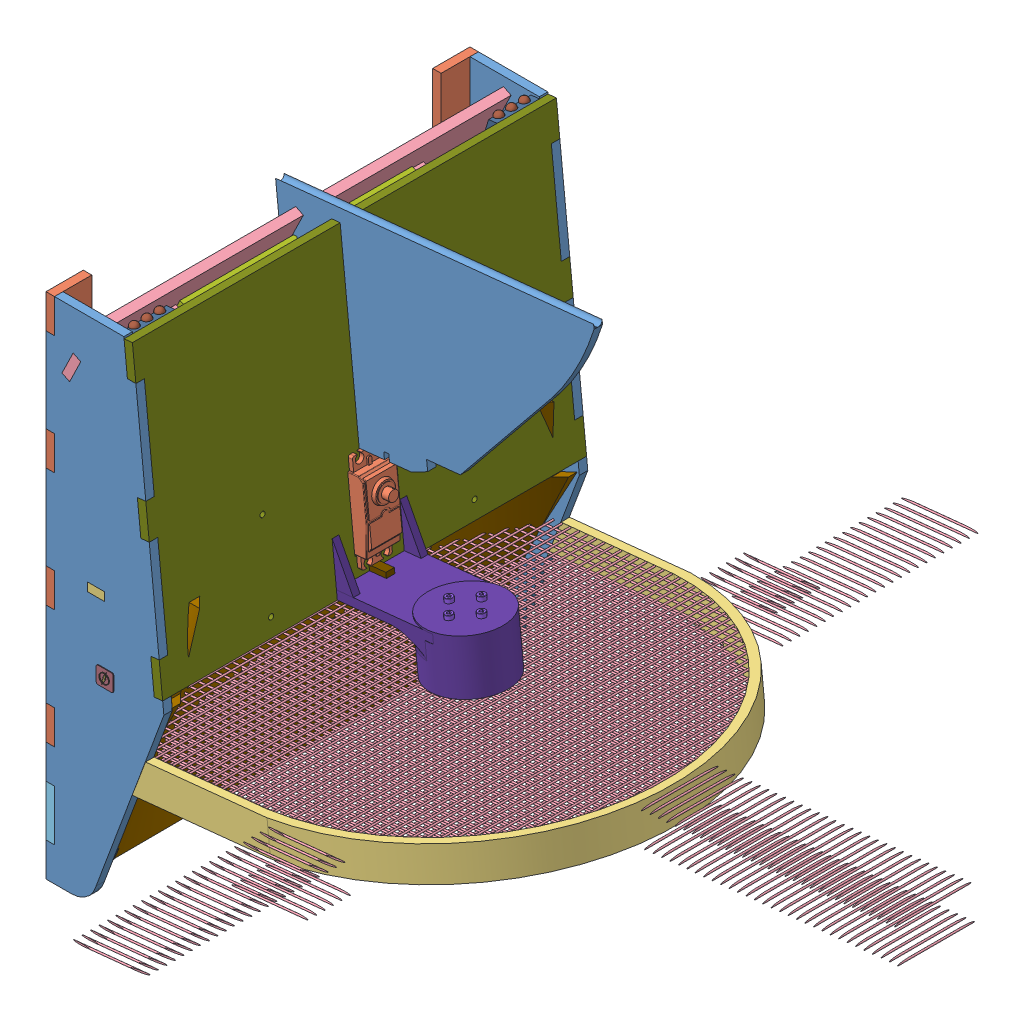
SolidWorks assembly AssStructSimu, configuration Défaut. Lengths in mm. (continued)
Components (placement in the parent): (continued)
- AssCarte-1: AssCarte [Défaut] at (38.0121 147.1029 290.772) x (-0.101852 0.9948 0) z (0.9948 0.101852 0) size (66.52 130.57 98.72) (hidden) (continued)
  - carte_onduleur_v3-1: carte_onduleur_v3 [Défaut] at (-131.8199 12.0892 20.7912) size (66.52 130.57 82.34) (continued)
    - C_DEC_COMP3-1: C_DEC_COMP3 [Défaut] at (-14.6 -22.9 0.803) x (0 -1 0) z (0 0 1) size (2.34 1.04 0.5) (continued)
      - Open CASCADE STEP translator 6.8 1.6.1-1: Open CASCADE STEP translator 6.8 1.6.1 [Défaut] at origin size (2.34 1.04 0.5) (continued)
        - Pin_2-1: Pin_2 [Défaut] at origin size (0.51 1.02 0.5)
    - D_VBAT-1: D_VBAT [Défaut] at (-1.2 46.4 0.803) x (0 -1 0) z (0 0 1) size (2.34 1.04 0.5)
      - Open CASCADE STEP translator 6.8 1.6.1-1: Open CASCADE STEP translator 6.8 1.6.1 [Défaut] at origin size (2.34 1.04 0.5)
        - Body_1-1: Body_1 [Défaut] at origin size (2.29 1.04 0.43)
        - Pin_1-1: Pin_1 [Défaut] at (0.3048 0 0) x (-1 0 0) z (0 0 1) size (0.51 1.02 0.5)
        - Pin_2-1: Pin_2 [Défaut] at origin size (0.51 1.02 0.5)
    - D_3V-1: D_3V [Défaut] at (1.3 46.3 0.803) x (0 -1 0) z (0 0 1) size (2.34 1.04 0.5)
      - Open CASCADE STEP translator 6.8 1.6.1-1: Open CASCADE STEP translator 6.8 1.6.1 [Défaut] at origin size (2.34 1.04 0.5)
        - Body_1-1: Body_1 [Défaut] at origin size (2.29 1.04 0.43)
        - Pin_1-1: Pin_1 [Défaut] at (0.3048 0 0) x (-1 0 0) z (0 0 1) size (0.51 1.02 0.5)
        - Pin_2-1: Pin_2 [Défaut] at origin size (0.51 1.02 0.5)
    - D_5V-1: D_5V [Défaut] at (-3.7 46.4 0.803) x (0 -1 0) z (0 0 1) size (2.34 1.04 0.5)
      - Open CASCADE STEP translator 6.8 1.6.1-1: Open CASCADE STEP translator 6.8 1.6.1 [Défaut] at origin size (2.34 1.04 0.5)
        - Body_1-1: Body_1 [Défaut] at origin size (2.29 1.04 0.43)
        - Pin_1-1: Pin_1 [Défaut] at (0.3048 0 0) x (-1 0 0) z (0 0 1) size (0.51 1.02 0.5)
        - Pin_2-1: Pin_2 [Défaut] at origin size (0.51 1.02 0.5)
    - R1_1-1: R1_1 [Défaut] at (-20.2 -36.1 0.803) x (-1 0 0) z (0 0 1) size (2.34 1.04 0.5)
      - Open CASCADE STEP translator 6.8 1.12.1-1: Open CASCADE STEP translator 6.8 1.12.1 [Défaut] at origin size (2.34 1.04 0.5)
        - Body_1_3-1: Body_1_3 [Défaut] at origin size (2.29 1.04 0.43)
        - Pin_1_2-1: Pin_1_2 [Défaut] at (0.3048 0 0) x (-1 0 0) z (0 0 1) size (0.51 1.02 0.5)
        - Pin_2_2-1: Pin_2_2 [Défaut] at origin size (0.51 1.02 0.5)
    - R1_2-1: R1_2 [Défaut] at (-15.5 -34.6 0.803) x (-1 0 0) z (0 0 1) size (2.34 1.04 0.5)
      - Open CASCADE STEP translator 6.8 1.12.1-1: Open CASCADE STEP translator 6.8 1.12.1 [Défaut] at origin size (2.34 1.04 0.5)
        - Body_1_3-1: Body_1_3 [Défaut] at origin size (2.29 1.04 0.43)
        - Pin_1_2-1: Pin_1_2 [Défaut] at (0.3048 0 0) x (-1 0 0) z (0 0 1) size (0.51 1.02 0.5)
        - Pin_2_2-1: Pin_2_2 [Défaut] at origin size (0.51 1.02 0.5)
    - R1_3-1: R1_3 [Défaut] at (-20.3 -39.9 0.803) x (-1 0 0) z (0 0 1) size (2.34 1.04 0.5)
      - Open CASCADE STEP translator 6.8 1.12.1-1: Open CASCADE STEP translator 6.8 1.12.1 [Défaut] at origin size (2.34 1.04 0.5)
        - Body_1_3-1: Body_1_3 [Défaut] at origin size (2.29 1.04 0.43)
        - Pin_1_2-1: Pin_1_2 [Défaut] at (0.3048 0 0) x (-1 0 0) z (0 0 1) size (0.51 1.02 0.5)
        - Pin_2_2-1: Pin_2_2 [Défaut] at origin size (0.51 1.02 0.5)
    - R1_4-1: R1_4 [Défaut] at (-20.3 -38.1 0.803) x (-1 0 0) z (0 0 1) size (2.34 1.04 0.5)
      - Open CASCADE STEP translator 6.8 1.12.1-1: Open CASCADE STEP translator 6.8 1.12.1 [Défaut] at origin size (2.34 1.04 0.5)
        - Body_1_3-1: Body_1_3 [Défaut] at origin size (2.29 1.04 0.43)
        - Pin_1_2-1: Pin_1_2 [Défaut] at (0.3048 0 0) x (-1 0 0) z (0 0 1) size (0.51 1.02 0.5)
        - Pin_2_2-1: Pin_2_2 [Défaut] at origin size (0.51 1.02 0.5)
    - R1_5-1: R1_5 [Défaut] at (-17.1336 -39.7 0.803) size (2.34 1.04 0.5)
      - Open CASCADE STEP translator 6.8 1.12.1-1: Open CASCADE STEP translator 6.8 1.12.1 [Défaut] at origin size (2.34 1.04 0.5)
        - Body_1_3-1: Body_1_3 [Défaut] at origin size (2.29 1.04 0.43)
        - Pin_1_2-1: Pin_1_2 [Défaut] at (0.3048 0 0) x (-1 0 0) z (0 0 1) size (0.51 1.02 0.5)
        - Pin_2_2-1: Pin_2_2 [Défaut] at origin size (0.51 1.02 0.5)
    - R2_1-1: R2_1 [Défaut] at (-18.5 -9.5 0.803) x (-1 0 0) z (0 0 1) size (2.34 1.04 0.5)
      - Open CASCADE STEP translator 6.8 1.12.1-1: Open CASCADE STEP translator 6.8 1.12.1 [Défaut] at origin size (2.34 1.04 0.5)
        - Body_1_3-1: Body_1_3 [Défaut] at origin size (2.29 1.04 0.43)
        - Pin_1_2-1: Pin_1_2 [Défaut] at (0.3048 0 0) x (-1 0 0) z (0 0 1) size (0.51 1.02 0.5)
        - Pin_2_2-1: Pin_2_2 [Défaut] at origin size (0.51 1.02 0.5)
    - R2_2-1: R2_2 [Défaut] at (-13.1 -8 0.803) x (-1 0 0) z (0 0 1) size (2.34 1.04 0.5)
      - Open CASCADE STEP translator 6.8 1.12.1-1: Open CASCADE STEP translator 6.8 1.12.1 [Défaut] at origin size (2.34 1.04 0.5)
        - Body_1_3-1: Body_1_3 [Défaut] at origin size (2.29 1.04 0.43)
        - Pin_1_2-1: Pin_1_2 [Défaut] at (0.3048 0 0) x (-1 0 0) z (0 0 1) size (0.51 1.02 0.5)
        - Pin_2_2-1: Pin_2_2 [Défaut] at origin size (0.51 1.02 0.5)
    - R2_3-1: R2_3 [Défaut] at (-18.5 -11.2 0.803) x (-1 0 0) z (0 0 1) size (2.34 1.04 0.5)
      - Open CASCADE STEP translator 6.8 1.12.1-1: Open CASCADE STEP translator 6.8 1.12.1 [Défaut] at origin size (2.34 1.04 0.5)
        - Body_1_3-1: Body_1_3 [Défaut] at origin size (2.29 1.04 0.43)
        - Pin_1_2-1: Pin_1_2 [Défaut] at (0.3048 0 0) x (-1 0 0) z (0 0 1) size (0.51 1.02 0.5)
        - Pin_2_2-1: Pin_2_2 [Défaut] at origin size (0.51 1.02 0.5)
    - R2_4-1: R2_4 [Défaut] at (-18.5 -12.8 0.803) x (-1 0 0) z (0 0 1) size (2.34 1.04 0.5)
      - Open CASCADE STEP translator 6.8 1.12.1-1: Open CASCADE STEP translator 6.8 1.12.1 [Défaut] at origin size (2.34 1.04 0.5)
        - Body_1_3-1: Body_1_3 [Défaut] at origin size (2.29 1.04 0.43)
        - Pin_1_2-1: Pin_1_2 [Défaut] at (0.3048 0 0) x (-1 0 0) z (0 0 1) size (0.51 1.02 0.5)
        - Pin_2_2-1: Pin_2_2 [Défaut] at origin size (0.51 1.02 0.5)
    - R2_5-1: R2_5 [Défaut] at (-15.1336 -13 0.803) size (2.34 1.04 0.5)
      - Open CASCADE STEP translator 6.8 1.12.1-1: Open CASCADE STEP translator 6.8 1.12.1 [Défaut] at origin size (2.34 1.04 0.5)
        - Body_1_3-1: Body_1_3 [Défaut] at origin size (2.29 1.04 0.43)
        - Pin_1_2-1: Pin_1_2 [Défaut] at (0.3048 0 0) x (-1 0 0) z (0 0 1) size (0.51 1.02 0.5)
        - Pin_2_2-1: Pin_2_2 [Défaut] at origin size (0.51 1.02 0.5)
    - R3_1-1: R3_1 [Défaut] at (-19.9 -23.1 0.803) x (-1 0 0) z (0 0 1) size (2.34 1.04 0.5)
      - Open CASCADE STEP translator 6.8 1.12.1-1: Open CASCADE STEP translator 6.8 1.12.1 [Défaut] at origin size (2.34 1.04 0.5)
        - Body_1_3-1: Body_1_3 [Défaut] at origin size (2.29 1.04 0.43)
        - Pin_1_2-1: Pin_1_2 [Défaut] at (0.3048 0 0) x (-1 0 0) z (0 0 1) size (0.51 1.02 0.5)
        - Pin_2_2-1: Pin_2_2 [Défaut] at origin size (0.51 1.02 0.5)
    - R3_2-1: R3_2 [Défaut] at (-14.7 -21.6 0.803) x (-1 0 0) z (0 0 1) size (2.34 1.04 0.5)
      - Open CASCADE STEP translator 6.8 1.12.1-1: Open CASCADE STEP translator 6.8 1.12.1 [Défaut] at origin size (2.34 1.04 0.5)
        - Body_1_3-1: Body_1_3 [Défaut] at origin size (2.29 1.04 0.43)
        - Pin_1_2-1: Pin_1_2 [Défaut] at (0.3048 0 0) x (-1 0 0) z (0 0 1) size (0.51 1.02 0.5)
        - Pin_2_2-1: Pin_2_2 [Défaut] at origin size (0.51 1.02 0.5)
    - R3_3-1: R3_3 [Défaut] at (-19.9 -24.8 0.803) x (-1 0 0) z (0 0 1) size (2.34 1.04 0.5)
      - Open CASCADE STEP translator 6.8 1.12.1-1: Open CASCADE STEP translator 6.8 1.12.1 [Défaut] at origin size (2.34 1.04 0.5)
        - Body_1_3-1: Body_1_3 [Défaut] at origin size (2.29 1.04 0.43)
        - Pin_1_2-1: Pin_1_2 [Défaut] at (0.3048 0 0) x (-1 0 0) z (0 0 1) size (0.51 1.02 0.5)
        - Pin_2_2-1: Pin_2_2 [Défaut] at origin size (0.51 1.02 0.5)
    - R3_4-1: R3_4 [Défaut] at (-19.9 -26.4 0.803) x (-1 0 0) z (0 0 1) size (2.34 1.04 0.5)
      - Open CASCADE STEP translator 6.8 1.12.1-1: Open CASCADE STEP translator 6.8 1.12.1 [Défaut] at origin size (2.34 1.04 0.5)
        - Body_1_3-1: Body_1_3 [Défaut] at origin size (2.29 1.04 0.43)
        - Pin_1_2-1: Pin_1_2 [Défaut] at (0.3048 0 0) x (-1 0 0) z (0 0 1) size (0.51 1.02 0.5)
        - Pin_2_2-1: Pin_2_2 [Défaut] at origin size (0.51 1.02 0.5)
    - R3_5-1: R3_5 [Défaut] at (-16.7336 -26.5 0.803) size (2.34 1.04 0.5)
      - Open CASCADE STEP translator 6.8 1.12.1-1: Open CASCADE STEP translator 6.8 1.12.1 [Défaut] at origin size (2.34 1.04 0.5)
        - Body_1_3-1: Body_1_3 [Défaut] at origin size (2.29 1.04 0.43)
        - Pin_1_2-1: Pin_1_2 [Défaut] at (0.3048 0 0) x (-1 0 0) z (0 0 1) size (0.51 1.02 0.5)
        - Pin_2_2-1: Pin_2_2 [Défaut] at origin size (0.51 1.02 0.5)
    - R_LED_3V3-1: R_LED_3V3 [Défaut] at (1.3 47.9 0.803) x (0 1 0) z (0 0 1) size (2.34 1.04 0.5)
      - Open CASCADE STEP translator 6.8 1.12.1-1: Open CASCADE STEP translator 6.8 1.12.1 [Défaut] at origin size (2.34 1.04 0.5)
        - Body_1_3-1: Body_1_3 [Défaut] at origin size (2.29 1.04 0.43)
        - Pin_1_2-1: Pin_1_2 [Défaut] at (0.3048 0 0) x (-1 0 0) z (0 0 1) size (0.51 1.02 0.5)
        - Pin_2_2-1: Pin_2_2 [Défaut] at origin size (0.51 1.02 0.5)
    - R_LED_5V-1: R_LED_5V [Défaut] at (-3.7 47.7 0.803) x (0 1 0) z (0 0 1) size (2.34 1.04 0.5)
      - Open CASCADE STEP translator 6.8 1.12.1-1: Open CASCADE STEP translator 6.8 1.12.1 [Défaut] at origin size (2.34 1.04 0.5)
        - Body_1_3-1: Body_1_3 [Défaut] at origin size (2.29 1.04 0.43)
        - Pin_1_2-1: Pin_1_2 [Défaut] at (0.3048 0 0) x (-1 0 0) z (0 0 1) size (0.51 1.02 0.5)
        - Pin_2_2-1: Pin_2_2 [Défaut] at origin size (0.51 1.02 0.5)
    - R_LED_VBAT-1: R_LED_VBAT [Défaut] at (-1.2 47.9 0.803) x (0 1 0) z (0 0 1) size (2.34 1.04 0.5)
      - Open CASCADE STEP translator 6.8 1.12.1-1: Open CASCADE STEP translator 6.8 1.12.1 [Défaut] at origin size (2.34 1.04 0.5)
        - Body_1_3-1: Body_1_3 [Défaut] at origin size (2.29 1.04 0.43)
        - Pin_1_2-1: Pin_1_2 [Défaut] at (0.3048 0 0) x (-1 0 0) z (0 0 1) size (0.51 1.02 0.5)
        - Pin_2_2-1: Pin_2_2 [Défaut] at origin size (0.51 1.02 0.5)
  - AssEntretoise-1: AssEntretoise [Défaut] at (-156.8199 -51.2976 37.1344) x (0 0 -1) z (1 0 0) size (58.24 7.29 7.81)
    - socket head cap screw 4762_din-1: socket head cap screw 4762_din [EN ISO 4762 M3 x 5 - 5N] at (-2.4967 0.5867 0) size (8 5.5 5.5)
    - hexagonal_spacer_MF_M3_H20_HEX5.5_FTD6_MTL6-1: hexagonal_spacer_MF_M3_H20_HEX5.5_FTD6_MTL6 [Défaut] at (48.3433 0.5867 0) x (0 0 1) z (-1 0 0) size (6.36 5.51 26)
    - hex nut style 1 gradeab_din-1: hex nut style 1 gradeab_din [Hexagon Nut ISO 4032 - M3 - W - N] at (53.3433 0.5867 0) x (0 0.943962 0.330053) z (-1 0 0) size (5.5 6.35 2.4)
    - hexagonal_spacer_MF_M3_H12_HEX5.5_FTD6_MTL6-2: hexagonal_spacer_MF_M3_H12_HEX5.5_FTD6_MTL6 [Défaut] at (27.0633 0.5867 0) x (0 0.248308 0.968681) z (-1 0 0) size (6.36 5.51 18)
    - hexagonal_spacer_MF_M3_H12_HEX5.5_FTD6_MTL6-3: hexagonal_spacer_MF_M3_H12_HEX5.5_FTD6_MTL6 [Défaut] at (13.7833 0.5867 0) x (0 0 1) z (-1 0 0) size (6.36 5.51 18)
  - AssEntretoise-2: AssEntretoise [Défaut] at (-156.8199 68.7024 37.1344) x (0 0 -1) z (1 0 0) size (58.24 7.29 7.81)
    - socket head cap screw 4762_din-1: socket head cap screw 4762_din [EN ISO 4762 M3 x 5 - 5N] at (-2.4967 0.5867 0) size (8 5.5 5.5)
    - hexagonal_spacer_MF_M3_H20_HEX5.5_FTD6_MTL6-1: hexagonal_spacer_MF_M3_H20_HEX5.5_FTD6_MTL6 [Défaut] at (48.3433 0.5867 0) x (0 0 1) z (-1 0 0) size (6.36 5.51 26)
    - hex nut style 1 gradeab_din-1: hex nut style 1 gradeab_din [Hexagon Nut ISO 4032 - M3 - W - N] at (53.3433 0.5867 0) x (0 0.943962 0.330053) z (-1 0 0) size (5.5 6.35 2.4)
    - hexagonal_spacer_MF_M3_H12_HEX5.5_FTD6_MTL6-2: hexagonal_spacer_MF_M3_H12_HEX5.5_FTD6_MTL6 [Défaut] at (27.0633 0.5867 0) x (0 0.248308 0.968681) z (-1 0 0) size (6.36 5.51 18)
    - hexagonal_spacer_MF_M3_H12_HEX5.5_FTD6_MTL6-3: hexagonal_spacer_MF_M3_H12_HEX5.5_FTD6_MTL6 [Défaut] at (13.7833 0.5867 0) x (0 0 1) z (-1 0 0) size (6.36 5.51 18)
  - AssEntretoise-3: AssEntretoise [Défaut] at (-106.8199 -51.2976 37.1344) x (0 0 -1) z (1 0 0) size (58.24 7.29 7.81)
    - socket head cap screw 4762_din-1: socket head cap screw 4762_din [EN ISO 4762 M3 x 5 - 5N] at (-2.4967 0.5867 0) size (8 5.5 5.5)
    - hexagonal_spacer_MF_M3_H20_HEX5.5_FTD6_MTL6-1: hexagonal_spacer_MF_M3_H20_HEX5.5_FTD6_MTL6 [Défaut] at (48.3433 0.5867 0) x (0 0 1) z (-1 0 0) size (6.36 5.51 26)
    - hex nut style 1 gradeab_din-1: hex nut style 1 gradeab_din [Hexagon Nut ISO 4032 - M3 - W - N] at (53.3433 0.5867 0) x (0 0.943962 0.330053) z (-1 0 0) size (5.5 6.35 2.4)
    - hexagonal_spacer_MF_M3_H12_HEX5.5_FTD6_MTL6-2: hexagonal_spacer_MF_M3_H12_HEX5.5_FTD6_MTL6 [Défaut] at (27.0633 0.5867 0) x (0 0.248308 0.968681) z (-1 0 0) size (6.36 5.51 18)
    - hexagonal_spacer_MF_M3_H12_HEX5.5_FTD6_MTL6-3: hexagonal_spacer_MF_M3_H12_HEX5.5_FTD6_MTL6 [Défaut] at (13.7833 0.5867 0) x (0 0 1) z (-1 0 0) size (6.36 5.51 18)
  - AssEntretoise-4: AssEntretoise [Défaut] at (-106.8199 68.7024 37.1344) x (0 0 -1) z (1 0 0) size (58.24 7.29 7.81)
    - socket head cap screw 4762_din-1: socket head cap screw 4762_din [EN ISO 4762 M3 x 5 - 5N] at (-2.4967 0.5867 0) size (8 5.5 5.5)
    - hexagonal_spacer_MF_M3_H20_HEX5.5_FTD6_MTL6-1: hexagonal_spacer_MF_M3_H20_HEX5.5_FTD6_MTL6 [Défaut] at (48.3433 0.5867 0) x (0 0 1) z (-1 0 0) size (6.36 5.51 26)
    - hex nut style 1 gradeab_din-1: hex nut style 1 gradeab_din [Hexagon Nut ISO 4032 - M3 - W - N] at (53.3433 0.5867 0) x (0 0.943962 0.330053) z (-1 0 0) size (5.5 6.35 2.4)
    - hexagonal_spacer_MF_M3_H12_HEX5.5_FTD6_MTL6-2: hexagonal_spacer_MF_M3_H12_HEX5.5_FTD6_MTL6 [Défaut] at (27.0633 0.5867 0) x (0 0.248308 0.968681) z (-1 0 0) size (6.36 5.51 18)
    - hexagonal_spacer_MF_M3_H12_HEX5.5_FTD6_MTL6-3: hexagonal_spacer_MF_M3_H12_HEX5.5_FTD6_MTL6 [Défaut] at (13.7833 0.5867 0) x (0 0 1) z (-1 0 0) size (6.36 5.51 18)
  - AssMpu-1: AssMpu [Défaut] at (-150.6881 40.5798 29.6372) x (0.908747 0.417347 0) z (0 0 1) size (8 8 22.28)
    - hex nut style 1 gradeab_din-1: hex nut style 1 gradeab_din [Hexagon Nut ISO 4032 - M3 - W - N] at (0.2783 0.3227 1.2) size (5.5 6.35 2.4)
    - plain washer 6903 type ab_din-1: plain washer 6903 type ab_din [DIN 6903-A3] at (0.2783 0.3227 1.2) x (0 0 1) z (-1 0 0) size (1 8 8)
    - socket head cap screw 4762_din-1: socket head cap screw 4762_din [EN ISO 4762 M3 x 5 - 5N] at (0.2783 0.3227 19.76) x (0 0 -1) z (-0.852155 0.523289 0) size (8 5.5 5.5)
    - hexagonal_spacer_MF_M3_H12_HEX5.5_FTD6_MTL6-1: hexagonal_spacer_MF_M3_H12_HEX5.5_FTD6_MTL6 [Défaut] at (0.2783 0.3227 3.48) size (6.36 5.51 18)
  - AssMpu-2: AssMpu [Défaut] at (-130.3481 40.6665 29.6372) size (8 8 22.28)
    - hex nut style 1 gradeab_din-1: hex nut style 1 gradeab_din [Hexagon Nut ISO 4032 - M3 - W - N] at (0.2783 0.3227 1.2) size (5.5 6.35 2.4)
    - plain washer 6903 type ab_din-1: plain washer 6903 type ab_din [DIN 6903-A3] at (0.2783 0.3227 1.2) x (0 0 1) z (-1 0 0) size (1 8 8)
    - socket head cap screw 4762_din-1: socket head cap screw 4762_din [EN ISO 4762 M3 x 5 - 5N] at (0.2783 0.3227 19.76) x (0 0 -1) z (-0.852155 0.523289 0) size (8 5.5 5.5)
    - hexagonal_spacer_MF_M3_H12_HEX5.5_FTD6_MTL6-1: hexagonal_spacer_MF_M3_H12_HEX5.5_FTD6_MTL6 [Défaut] at (0.2783 0.3227 3.48) size (6.36 5.51 18)
  - AssCosse-1: AssCosse [Défaut] at (-142.6764 26.8797 71.168) x (0 -1 0) z (-0.344896 0 -0.938641) size (9.83 18.66 11.64)
    - socket head cap screw 4762_din-1: socket head cap screw 4762_din [EN ISO 4762 M3 x 6 - 6N] at (-5.1064 0.3659 0) size (9 5.5 5.5)
    - plain washer 6903 type ab_din-1: plain washer 6903 type ab_din [DIN 6903-A3] at (-2.1064 0.3659 0) size (1 8 8)
    - hex nut style 1 gradeab_din-2: hex nut style 1 gradeab_din [Hexagon Nut ISO 4032 - M3 - W - N] at (1.281 0.3659 0) x (0 0.924225 0.381849) z (-1 0 0) size (5.5 6.35 2.4)
    - 31880-1: 31880 [Default] at (0.4936 0.3659 0) x (0 0.344896 -0.938641) z (0 -0.938641 -0.344896) size (5.54 5 17.37)
  - AssCosse-2: AssCosse [Défaut] at (-142.6764 -2.9203 71.168) x (0 -1 0) z (-0.344896 0 -0.938641) size (9.83 18.66 11.64)
    - socket head cap screw 4762_din-1: socket head cap screw 4762_din [EN ISO 4762 M3 x 6 - 6N] at (-5.1064 0.3659 0) size (9 5.5 5.5)
    - plain washer 6903 type ab_din-1: plain washer 6903 type ab_din [DIN 6903-A3] at (-2.1064 0.3659 0) size (1 8 8)
    - hex nut style 1 gradeab_din-2: hex nut style 1 gradeab_din [Hexagon Nut ISO 4032 - M3 - W - N] at (1.281 0.3659 0) x (0 0.924225 0.381849) z (-1 0 0) size (5.5 6.35 2.4)
    - 31880-1: 31880 [Default] at (0.4936 0.3659 0) x (0 0.344896 -0.938641) z (0 -0.938641 -0.344896) size (5.54 5 17.37)
  - AssCosse-3: AssCosse [Défaut] at (-142.6764 12.0797 71.168) x (0 -1 0) z (-0.344896 0 -0.938641) size (9.83 18.66 11.64)
    - socket head cap screw 4762_din-1: socket head cap screw 4762_din [EN ISO 4762 M3 x 6 - 6N] at (-5.1064 0.3659 0) size (9 5.5 5.5)
    - plain washer 6903 type ab_din-1: plain washer 6903 type ab_din [DIN 6903-A3] at (-2.1064 0.3659 0) size (1 8 8)
    - hex nut style 1 gradeab_din-2: hex nut style 1 gradeab_din [Hexagon Nut ISO 4032 - M3 - W - N] at (1.281 0.3659 0) x (0 0.924225 0.381849) z (-1 0 0) size (5.5 6.35 2.4)
    - 31880-1: 31880 [Default] at (0.4936 0.3659 0) x (0 0.344896 -0.938641) z (0 -0.938641 -0.344896) size (5.54 5 17.37)
  - Terminal_QD_Female-1: Terminal_QD_Female [Default] at (-137.2199 31.5422 53.3942) x (0 1 0) z (-1 0 0) size (9.4 5.5 22.35)
  - Terminal_QD_Female-2: Terminal_QD_Female [Default] at (-137.3199 31.5422 36.2942) x (0 -1 0) z (-1 0 0) size (9.4 5.5 22.35)
  - Terminal_QD_Female-3: Terminal_QD_Female [Default] at (-137.2199 1.7422 53.3942) x (0 1 0) z (-1 0 0) size (9.4 5.5 22.35)
  - Terminal_QD_Female-4: Terminal_QD_Female [Default] at (-137.3199 1.7422 35.9942) x (0 1 0) z (-1 0 0) size (9.4 5.5 22.35)
  - Terminal_QD_Female-5: Terminal_QD_Female [Default] at (-137.3199 16.7422 35.9942) x (0 1 0) z (-1 0 0) size (9.4 5.5 22.35)
  - Terminal_QD_Female-6: Terminal_QD_Female [Default] at (-137.2199 16.7422 53.3942) x (0 1 0) z (-1 0 0) size (9.4 5.5 22.35)
- AssGoPro-1: AssGoPro [Défaut] at (4.1252 -17.5988 306.3631) x (0 0 1) z (-0.094708 0.995505 0) size (64.3 52.3 34.42)
  - GoPRo Frame for LCD Screen-1: GoPRo Frame for LCD Screen [Défaut] at (-2.6935 10.9558 5.5635) size (64.3 59.3 34.42)
    - GoProFrame MJM-1: GoProFrame MJM [Défaut] at (-3.6084 -1.6692 52.45) size (64.3 59.3 23.5)
    - GoPro Hero 3 Front Panel-1: GoPro Hero 3 Front Panel [Défaut] at (-3.6084 -1.6692 55.7) x (-1 0 0) z (0 0 -1) size (59.25 41.2 1.9)
    - GoPro Hero 3 Screen-1: GoPro Hero 3 Screen [Défaut] at (12.7166 3.9308 54.9) size (15 18 1)
    - GoPro Hero 3 Mode Button-1: GoPro Hero 3 Mode Button [Défaut] at (13.4166 -12.4692 54.95) x (-1 0 0) z (0 0 -1) size (11.97 12.11 3.03)
    - GoPro Hero 3 LED Cover-1: GoPro Hero 3 LED Cover [Défaut] at (3.1166 -9.3192 54.85) x (-0.999988 0.004848 0) z (0 0 -1) size (5 5 1.4)
    - GoPro Hero 3 LED Cover-2: GoPro Hero 3 LED Cover [Défaut] at (3.1166 -16.0692 54.85) x (-0.999988 0.004848 0) z (0 0 -1) size (5 5 1.4)
    - GoPro Hero 3 Housing-1: GoPro Hero 3 Housing [Défaut] at (-3.6084 -1.6692 55.7) size (59.37 41.3 29.84)
    - GoPro Hero 3 Lens-1: GoPro Hero 3 Lens [Défaut] at (-18.9334 5.6308 47.35) x (-0.380542 -0.924764 0) z (0 0 -1) size (13.71 15.7 7.94)
    - GoPro Hero 3 Indicator Cover-1: GoPro Hero 3 Indicator Cover [Défaut] at (-25.5834 -22.2692 69.9) x (-0.997412 0 -0.0719) z (0 1 0) size (3 3 2)
    - GoPro Hero 3 Indicator Cover-2: GoPro Hero 3 Indicator Cover [Défaut] at (-28.8834 12.2308 73) x (-0.999992 0.004018 0) z (0 0 1) size (3 3 2)
    - GoPro Hero 3 Indicator Cover-3: GoPro Hero 3 Indicator Cover [Défaut] at (20.6666 16.9308 58.4) x (-0.997739 0 -0.067212) z (0 1 0) size (3 3 2)
    - slot-1: slot [Défaut] at (-24.7434 -9.7363 65.05) x (0 1 0) z (0 0 -1) size (16 15.02 2.44)
    - GoPro Hero 3 HDMI pin-1: GoPro Hero 3 HDMI pin [Défaut] at (-26.982 2.9815 24.7172) x (0.105491 0.98175 -0.158237) z (-0.992872 0.095109 -0.071829) size (3.29 0.86 3.28)
  - support1-2: support1 [Défaut] at (-1.3019 -18.8633 67.0135) x (0 0 1) z (-1 0 0) size (5 5 10)
Mates (geometry in assembly coordinates):
- Coïncidente3: coincident anti-aligned: plane of AssBase-1/AssG-1/P1-1 through (30.985 56.5967 180.0612) normal (-0.101852 0.9948 0); plane of AssToitMot-1/AssToit-1/P8-1 through (35.959 57.1059 175.0612) normal (0.101852 -0.9948 0)
- Coïncidente4: coincident anti-aligned: plane of AssBase-1/AssG-1/P1-1 through (28.948 76.4927 180.0612) normal (0.9948 0.101852 0); plane of AssToitMot-1/AssToit-1/P8-1 through (19.4248 169.5064 300.0612) normal (-0.9948 -0.101852 0)
- Coïncidente5: coincident aligned: plane of AssBase-1/AssG-1/P1-1 through (-9.9345 -130.354 175.0612) normal (0 0 -1); plane of AssToitMot-1/AssToit-1/P8-1 through (41.8155 -0.095 175.0612) normal (0 0 -1)
- Distance2: distance = 35 mm anti-aligned: plane of AssProtec-1/protec3c-1 through (95.0117 -49.9361 300.0612) normal (-0.101852 0.9948 0); plane of AssToitMot-1/AssToit-1/P8-1 through (43.8525 -19.991 175.0612) normal (0.101852 -0.9948 0)
- Coïncidente9: coincident: plane of AssBase-1/AssG-1/P1-1 through (44.5655 -26.9546 180.0612) normal (0.936958 -0.349442 0); line of AssProtec-1/protec3c-1 through (25.8557 -77.1211 180.0612) axis (0 0 -1)
- Coïncidente10: coincident aligned: plane of AssBase-1/AssG-1/P1-1 through (-9.9345 -130.354 175.0612) normal (0 0 -1); plane of AssProtec-1/protec3c-1 through (25.8557 -77.1211 175.0612) normal (0 0 -1)
- Coaxiale1: concentric aligned: cylinder of AssToitMot-1/AssToit-1/P8-1 through (32.7674 39.1877 240.0612) axis (0.9948 0.101852 0) radius 1.5; cylinder of AssCarte-1/AssEntretoise-3/hexagonal_spacer_MF_M3_H20_HEX5.5_FTD6_MTL6-1 through (31.9506 39.1041 240.0612) axis (0.9948 0.101852 0) radius 1.5
- Coïncidente11: coincident anti-aligned: plane of AssToitMot-1/AssToit-1/P8-1 through (24.3988 170.0157 300.0612) normal (0.9948 0.101852 0); plane of AssCarte-1/AssEntretoise-3/hexagonal_spacer_MF_M3_H20_HEX5.5_FTD6_MTL6-1 through (37.7414 39.6969 240.0612) normal (-0.9948 -0.101852 0)
- Coaxiale2: concentric aligned: cylinder of AssToitMot-1/AssToit-1/P8-1 through (37.86 -10.5523 360.0612) axis (0.9948 0.101852 0) radius 1.5; cylinder of AssCarte-1/AssEntretoise-2/hexagonal_spacer_MF_M3_H20_HEX5.5_FTD6_MTL6-1 through (37.0432 -10.6359 360.0612) axis (0.9948 0.101852 0) radius 1.5
- Coaxiale3: concentric aligned: cylinder of AssBase-1/socket head cap screw 4762_din-7 through (-18.7481 50.0525 255.3112) axis (0 0 -1) radius 1.5; cylinder of AssGoPro-1/support1-2 through (-18.7481 50.0525 305.0612) axis (0 0 -1) radius 1.5
- Coïncidente13: coincident anti-aligned: plane of AssBase-1/support2-1 through (-16.2048 52.5085 295.0612) normal (0 0 1); plane of AssGoPro-1/support1-2 through (-21.0001 47.327 295.0612) normal (0 0 -1)
